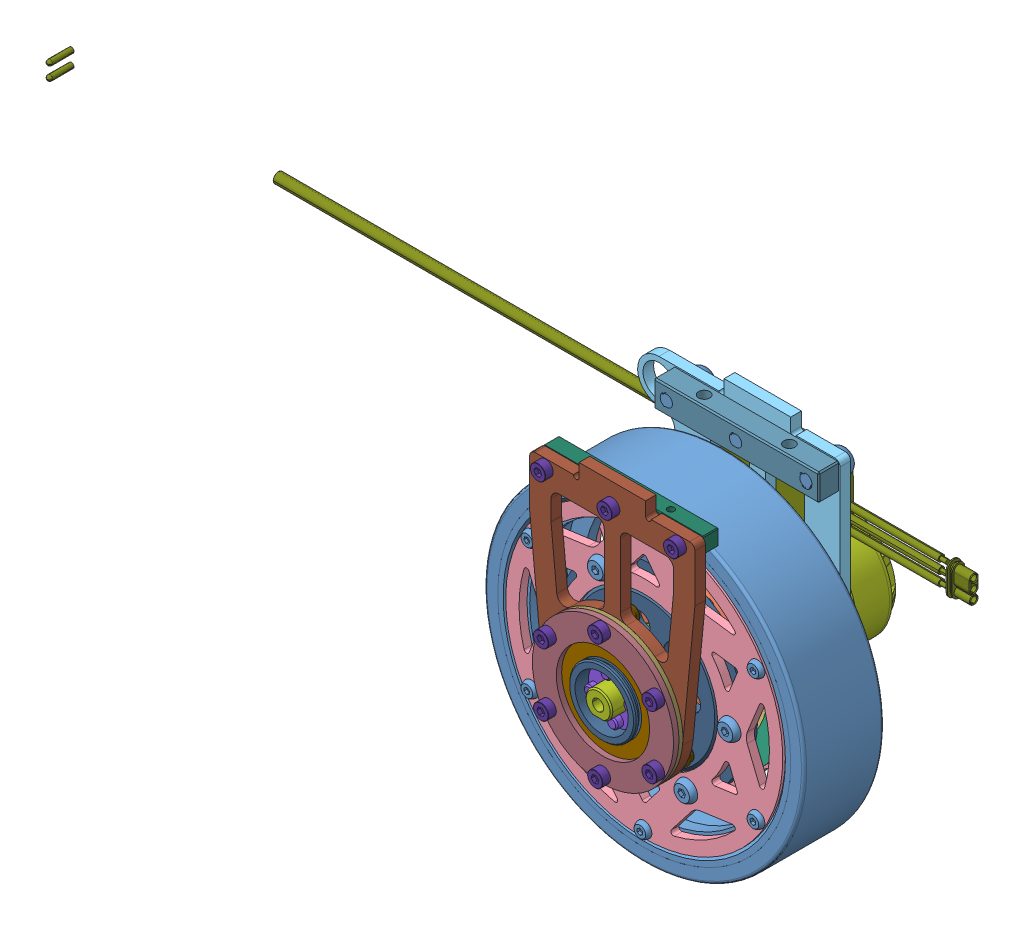
SolidWorks assembly 驱动轮部分, configuration 默认. Lengths in mm.
Overall size (142.07 142.07 99.6).
53 component instances, 19 part files, 115 mates.
Components (placement in the parent):
- 铝芯包胶轮-1: 铝芯包胶轮 [默认] at origin size (120 120 30)
- 3508电机座-1: 3508电机座 [默认] at (0 0 -27.5) x (1 0 0) z (0 -1 0) size (62 39.5 60.69)
- 薄型滚珠轴承6809zz45×58×7-1: 薄型滚珠轴承6809zz45×58×7 [默认] at (0 0 -12) x (0.929394 0.369089 0) z (0.369089 -0.929394 0) size (58 7 58)
- 舵轮盖板-内-1: 舵轮盖板-内 [内 ] at (0 0 -12) x (-0.5 -0.866025 0) z (0.866025 -0.5 0) size (104 3 104)
- 舵轮系基板-1: 舵轮系基板 [默认] at (0 0 -31.5) size (76 100.33 4)
- 舵轮系内侧轴承座-1: 舵轮系内侧轴承座 [默认] at (0 0 -5) x (0.5 0.866025 0) z (-0.866025 0.5 0) size (72 8 72)
- RoboMaster M3508直流无刷减速电机-1: RoboMaster M3508直流无刷减速电机 [默认] at (5.259 17.5861 -81.441) x (-0.925598 0.378508 0) z (0 0 1) size (42 42.01 98.4)
- 舵轮盖板-内-2: 舵轮盖板-内 [外] at (0 0 15) x (-0.5 -0.866025 0) z (0.866025 -0.5 0) size (104 3 104)
- 涨紧套Z21-10x20x13-1: 涨紧套Z21-10x20x13 [默认] at (0 0 13) x (0.985721 0.168386 0) z (0.168386 -0.985721 0) size (20 15.5 20)
- 法兰轴承-1: 法兰轴承 [25*37*7-1.5] at (0 0 28.5) x (0.417782 -0.908547 0) z (0.908547 0.417782 0) size (40 7 40)
- 轮组双端支撑件-1: 轮组双端支撑件 [默认] at (0 0 8) x (0.995882 0.09066 0) z (0.09066 -0.995882 0) size (70.95 23 70.95)
- 双端支撑板-1: 双端支撑板 [默认] at (0 0 23) size (62 96.5 4)
- 舵轮打印件垫片-1: 舵轮打印件垫片 [默认] at (0 0 27) size (53 53 1.5)
- 轮组压板-1: 轮组压板 [默认] at (0 0 28.5) size (53 53 2)
- 舵轮铝条直角连接件-2: 舵轮铝条直角连接件 [默认] at (0 60 -23.5) size (62 10 8)
- 双端支撑铝条-1: 双端支撑铝条 [默认] at (0 62 20) size (60 6 6)
- C620无刷电机调速器-1: C620无刷电机调速器 [默认] at (1.7 41 -36.9) x (1 0 0) z (0 -1 0) size (59.4 11.5 26.13)
- 12.9级圆柱头螺钉-4: 12.9级圆柱头螺钉 [M3*10] at (25 62 30) x (0.999644 -0.026698 0) z (0 0 1) size (5.68 5.68 13)
- 12.9级圆柱头螺钉-5: 12.9级圆柱头螺钉 [M3*10] at (0 62 30) x (0.999644 -0.026698 0) z (0 0 1) size (5.68 5.68 13)
- 12.9级圆柱头螺钉-6: 12.9级圆柱头螺钉 [M3*10] at (-25 62 30) x (0.999644 -0.026698 0) z (0 0 1) size (5.68 5.68 13)
- 12.9级圆柱头螺钉-7: 12.9级圆柱头螺钉 [M3*12] at (-20.3516 11.75 33.5) x (0.999644 -0.026698 0) z (0 0 1) size (5.68 5.68 15)
- 百瑞特防滑螺母-1: 百瑞特防滑螺母 [M3] at (-20.3516 11.75 20.6) x (0.875007 -0.48411 0) z (-0.48411 -0.875007 0) size (5.5 3.9 6.35)
- 12.9级圆柱头螺钉-8: 12.9级圆柱头螺钉 [M3*12] at (-20.3516 -11.75 33.5) x (0.991232 0.132136 0) z (0 0 1) size (5.68 5.68 15)
- 百瑞特防滑螺母-2: 百瑞特防滑螺母 [M3] at (-20.3516 -11.75 20.6) x (0.940696 -0.339252 0) z (-0.339252 -0.940696 0) size (5.5 3.9 6.35)
- 12.9级圆柱头螺钉-9: 12.9级圆柱头螺钉 [M3*12] at (0 -23.5 33.5) x (0.966338 0.257276 0) z (0 0 1) size (5.68 5.68 15)
- 百瑞特防滑螺母-3: 百瑞特防滑螺母 [M3] at (0 -23.5 20.6) x (0.976236 -0.216709 0) z (-0.216709 -0.976236 0) size (5.5 3.9 6.35)
- 12.9级圆柱头螺钉-10: 12.9级圆柱头螺钉 [M3*12] at (20.3516 -11.75 33.5) x (0.93815 0.34623 0) z (0 0 1) size (5.68 5.68 15)
- 百瑞特防滑螺母-4: 百瑞特防滑螺母 [M3] at (20.3516 -11.75 20.6) x (0.992186 -0.124769 0) z (-0.124769 -0.992186 0) size (5.5 3.9 6.35)
- 12.9级圆柱头螺钉-11: 12.9级圆柱头螺钉 [M3*12] at (20.3516 11.75 33.5) x (0.91791 0.396788 0) z (0 0 1) size (5.68 5.68 15)
- 百瑞特防滑螺母-5: 百瑞特防滑螺母 [M3] at (20.3516 11.75 20.6) x (0.997507 -0.07057 0) z (-0.07057 -0.997507 0) size (5.5 3.9 6.35)
- 12.9级圆柱头螺钉-12: 12.9级圆柱头螺钉 [M3*12] at (0 23.5 33.5) x (0.914007 0.405699 0) z (0 0 1) size (5.68 5.68 15)
- 百瑞特防滑螺母-6: 百瑞特防滑螺母 [M3] at (0 23.5 20.6) x (0.998146 -0.060863 0) z (-0.060863 -0.998146 0) size (5.5 3.9 6.35)
- 12.9级圆柱头螺钉-14: 12.9级圆柱头螺钉 [M4*10] at (19.4454 -19.4454 -35.5) x (-0.999764 -0.021708 0) z (0 0 -1) size (7.22 7.22 14)
- 12.9级圆柱头螺钉-15: 12.9级圆柱头螺钉 [M4*10] at (27.5 0 -35.5) x (-0.999764 -0.021708 0) z (0 0 -1) size (7.22 7.22 14)
- 12.9级圆柱头螺钉-16: 12.9级圆柱头螺钉 [M4*10] at (19.4454 19.4454 -35.5) x (-0.999764 -0.021708 0) z (0 0 -1) size (7.22 7.22 14)
- 12.9级圆柱头螺钉-17: 12.9级圆柱头螺钉 [M4*10] at (-19.4454 -19.4454 -35.5) x (-0.999764 -0.021708 0) z (0 0 -1) size (7.22 7.22 14)
- 12.9级圆柱头螺钉-18: 12.9级圆柱头螺钉 [M4*10] at (-27.5 0 -35.5) x (-0.999764 -0.021708 0) z (0 0 -1) size (7.22 7.22 14)
- 12.9级圆柱头螺钉-19: 12.9级圆柱头螺钉 [M4*10] at (-19.4454 19.4454 -35.5) x (-0.999764 -0.021708 0) z (0 0 -1) size (7.22 7.22 14)
- 10.9级半圆头螺栓-1: 10.9级半圆头螺栓 [M5*12] at (-26 60 -31.5) x (0.059849 -0.998207 0) z (-0.998207 -0.059849 0) size (9.5 14.75 9.5)
- 10.9级半圆头螺栓-2: 10.9级半圆头螺栓 [M5*12] at (26 60 -31.5) x (0.059849 -0.998207 0) z (-0.998207 -0.059849 0) size (9.5 14.75 9.5)
- 10.9级半圆头螺栓-3: 10.9级半圆头螺栓 [M5*12] at (0 60 -31.5) x (0.059849 -0.998207 0) z (-0.998207 -0.059849 0) size (9.5 14.75 9.5)
- 10.9级半圆头螺栓-4: 10.9级半圆头螺栓 [M4*8] at (-16.25 -28.1458 15) x (0.975246 0.221124 0) z (-0.221124 0.975246 0) size (7.6 10.2 7.6)
- 10.9级半圆头螺栓-5: 10.9级半圆头螺栓 [M4*8] at (16.25 -28.1458 15) x (0.975246 0.221124 0) z (-0.221124 0.975246 0) size (7.6 10.2 7.6)
- 10.9级半圆头螺栓-6: 10.9级半圆头螺栓 [M4*8] at (32.5 0 15) x (0.975246 0.221124 0) z (-0.221124 0.975246 0) size (7.6 10.2 7.6)
- 10.9级半圆头螺栓-7: 10.9级半圆头螺栓 [M4*8] at (16.25 28.1458 15) x (0.92785 0.372955 0) z (-0.372955 0.92785 0) size (7.6 10.2 7.6)
- 10.9级半圆头螺栓-8: 10.9级半圆头螺栓 [M4*8] at (-16.25 28.1458 15) x (0.872808 0.488064 0) z (-0.488064 0.872808 0) size (7.6 10.2 7.6)
- 10.9级半圆头螺栓-9: 10.9级半圆头螺栓 [M4*8] at (-32.5 0 15) x (0.823514 0.567296 0) z (-0.567296 0.823514 0) size (7.6 10.2 7.6)
- 10.9级半圆头螺栓-11: 10.9级半圆头螺栓 [M3*8] at (-42.4352 24.5 15) x (0.243917 0.969796 0) z (-0.969796 0.243917 0) size (5.7 9.65 5.7)
- 10.9级半圆头螺栓-13: 10.9级半圆头螺栓 [M3*8] at (-42.4352 -24.5 15) x (0.087067 0.996202 0) z (-0.996202 0.087067 0) size (5.7 9.65 5.7)
- 10.9级半圆头螺栓-14: 10.9级半圆头螺栓 [M3*8] at (0 -49 15) x (-0.04049 0.99918 0) z (-0.99918 -0.04049 0) size (5.7 9.65 5.7)
- 10.9级半圆头螺栓-15: 10.9级半圆头螺栓 [M3*8] at (42.4352 -24.5 15) x (-0.133449 0.991056 0) z (-0.991056 -0.133449 0) size (5.7 9.65 5.7)
- 10.9级半圆头螺栓-16: 10.9级半圆头螺栓 [M3*8] at (42.4352 24.5 15) x (-0.187203 0.982321 0) z (-0.982321 -0.187203 0) size (5.7 9.65 5.7)
- 10.9级半圆头螺栓-17: 10.9级半圆头螺栓 [M3*8] at (0 49 15) x (-0.19675 0.980454 0) z (-0.980454 -0.19675 0) size (5.7 9.65 5.7)
Mates (geometry in assembly coordinates):
- 同心1: concentric aligned: cylinder of 铝芯包胶轮-1 through (0 0 12) axis (0 0 1) radius 52; cylinder of 舵轮盖板-内-1 through (0 0 -15) axis (0 0 1) radius 27.5
- 重合1: coincident anti-aligned: plane of 铝芯包胶轮-1 through (0 0 -12) normal (0 0 -1); plane of 舵轮盖板-内-1 through (0 0 -12) normal (0 0 1)
- 同心2: concentric aligned: cylinder of 铝芯包胶轮-1 through (-42.4352 24.5 12) axis (0 0 1) radius 1.25; cylinder of 舵轮盖板-内-1 through (-42.4352 24.5 -15) axis (0 0 1) radius 1.525
- 同心3: concentric anti-aligned: cylinder of 3508电机座-1 through (0 0 -27.5) axis (0 0 -1) radius 22.5; cylinder of 舵轮盖板-内-1 through (0 0 -15) axis (0 0 1) radius 27.5
- 同心4: concentric aligned: cylinder of 3508电机座-1 through (0 0 -27.5) axis (0 0 -1) radius 22.5; cylinder of 薄型滚珠轴承6809zz45×58×7-1 through (0 0 -5) axis (0 0 -1) radius 22.5
- 重合2: coincident anti-aligned: plane of 3508电机座-1 through (-24 0 -12) normal (0 0 1); plane of 薄型滚珠轴承6809zz45×58×7-1 through (0 0 -12) normal (0 0 -1)
- 重合3: coincident anti-aligned: plane of 薄型滚珠轴承6809zz45×58×7-1 through (0 0 -12) normal (0 0 -1); plane of 舵轮盖板-内-1 through (0 0 -12) normal (0 0 1)
- 平行1: parallel aligned: plane of 舵轮系基板-1 through (31 65 -27.5) normal (1 0 0)
- 同心5: concentric aligned: cylinder of 3508电机座-1 through (0 0 -27.5) axis (0 0 -1) radius 24; cylinder of 舵轮系基板-1 through (0 0 -27.5) axis (0 0 -1) radius 24
- 重合4: coincident anti-aligned: plane of 3508电机座-1 through (-31 0 -27.5) normal (0 0 -1); plane of 舵轮系基板-1 through (0 0 -27.5) normal (0 0 1)
- 同心6: concentric anti-aligned: cylinder of 薄型滚珠轴承6809zz45×58×7-1 through (0 0 -5) axis (0 0 -1) radius 29; cylinder of 舵轮系内侧轴承座-1 through (0 0 -12) axis (0 0 1) radius 36
- 重合5: coincident anti-aligned: plane of 薄型滚珠轴承6809zz45×58×7-1 through (0 0 -5) normal (0 0 1); plane of 舵轮系内侧轴承座-1 through (0 0 -5) normal (0 0 -1)
- 同心7: concentric anti-aligned: cylinder of 舵轮盖板-内-1 through (16.25 28.1458 -15) axis (0 0 1) radius 2; cylinder of 舵轮系内侧轴承座-1 through (16.25 28.1458 -12) axis (0 0 -1) radius 1.65
- 同心9: concentric anti-aligned: cylinder of 3508电机座-1 through (19.4454 -19.4454 -22.5) axis (0 0 1) radius 1.65; cylinder of 舵轮系基板-1 through (19.4454 -19.4454 -27.5) axis (0 0 -1) radius 2
- 同心10: concentric aligned: cylinder of 3508电机座-1 through (0 0 -27.5) axis (0 0 -1) radius 21; cylinder of RoboMaster M3508直流无刷减速电机-1 through (0 0 -31) axis (0 0 -1) radius 21
- 重合6: coincident anti-aligned: plane of 3508电机座-1 through (-21 0 5) normal (0 0 -1); plane of RoboMaster M3508直流无刷减速电机-1 through (9.1924 9.1924 5) normal (0 0 1)
- 同心11: concentric aligned: cylinder of 3508电机座-1 through (0 17.5 8) axis (0 0 1) radius 2; cylinder of RoboMaster M3508直流无刷减速电机-1 through (0 17.5 5) axis (0 0 1) radius 1.65
- 同心12: concentric aligned: cylinder of RoboMaster M3508直流无刷减速电机-1 through (0 0 32.3) axis (0 0 1) radius 5; cylinder of 舵轮盖板-内-2 through (0 0 12) axis (0 0 1) radius 27.5
- 重合7: coincident anti-aligned: plane of 铝芯包胶轮-1 through (0 0 12) normal (0 0 1); plane of 舵轮盖板-内-2 through (0 0 12) normal (0 0 -1)
- 同心13: concentric aligned: cylinder of 铝芯包胶轮-1 through (0 49 12) axis (0 0 1) radius 1.25; cylinder of 舵轮盖板-内-2 through (0 49 12) axis (0 0 1) radius 1.525
- 同心14: concentric anti-aligned: cylinder of RoboMaster M3508直流无刷减速电机-1 through (0 0 32.3) axis (0 0 1) radius 5; cylinder of 涨紧套Z21-10x20x13-1 through (0 0 26) axis (0 0 -1) radius 5
- 同心15: concentric anti-aligned: cylinder of 涨紧套Z21-10x20x13-1 through (0 0 26) axis (0 0 -1) radius 10; cylinder of 法兰轴承-1 through (0 0 21.5) axis (0 0 1) radius 12.5
- 重合8: coincident anti-aligned: plane of 舵轮盖板-内-2 through (0 0 12) normal (0 0 -1); plane of 轮组双端支撑件-1 through (-27.3619 -2.4909 12) normal (0 0 1)
- 同心16: concentric anti-aligned: cylinder of RoboMaster M3508直流无刷减速电机-1 through (0 0 32.3) axis (0 0 1) radius 5; cylinder of 轮组双端支撑件-1 through (0 0 8) axis (0 0 -1) radius 12.5
- 距离1: distance = 5 mm aligned: plane of 涨紧套Z21-10x20x13-1 through (0 0 26) normal (0 0 1); plane of 轮组双端支撑件-1 through (-9.9588 -0.9066 31) normal (0 0 1)
- 重合9: coincident aligned: plane of 法兰轴承-1 through (0 0 28.5) normal (0 0 1); plane of 轮组双端支撑件-1 through (11.5522 1.0517 28.5) normal (0 0 1)
- 重合10: coincident anti-aligned: plane of 法兰轴承-1 through (0 0 27) normal (0 0 -1); plane of 双端支撑板-1 through (0 0 27) normal (0 0 1)
- 同心17: concentric anti-aligned: cylinder of 法兰轴承-1 through (0 0 21.5) axis (0 0 1) radius 18.5; cylinder of 双端支撑板-1 through (0 0 27) axis (0 0 -1) radius 18.5
- 平行2: parallel aligned: plane of 舵轮系基板-1 through (-31 0 -27.5) normal (-1 0 0); plane of 双端支撑板-1 through (-31 0 27) normal (-1 0 0)
- 同心18: concentric anti-aligned: cylinder of 法兰轴承-1 through (0 0 27) axis (0 0 1) radius 20; cylinder of 舵轮打印件垫片-1 through (0 0 28.5) axis (0 0 -1) radius 20.5
- 重合11: coincident anti-aligned: plane of 双端支撑板-1 through (0 0 27) normal (0 0 1); plane of 舵轮打印件垫片-1 through (0 0 27) normal (0 0 -1)
- 重合12: coincident aligned: plane of 舵轮打印件垫片-1 through (0 0 27) normal (0 1 0)
- 重合13: coincident anti-aligned: plane of 舵轮打印件垫片-1 through (0 0 28.5) normal (0 0 1); plane of 轮组压板-1 through (0 0 28.5) normal (0 0 -1)
- 同心19: concentric aligned: cylinder of 轮组双端支撑件-1 through (0 0 8) axis (0 0 -1) radius 10; cylinder of 轮组压板-1 through (0 0 30.5) axis (0 0 -1) radius 17.5
- 同心20: concentric aligned: cylinder of 舵轮打印件垫片-1 through (0 23.5 27) axis (0 0 1) radius 1.65; cylinder of 轮组压板-1 through (0 23.5 28.5) axis (0 0 1) radius 1.525
- 重合15: coincident anti-aligned: plane of 舵轮系基板-1 through (0 0 -27.5) normal (0 0 1); plane of 舵轮铝条直角连接件-2 through (0 60 -27.5) normal (0 0 -1)
- 同心22: concentric anti-aligned: cylinder of 舵轮系基板-1 through (26 60 -27.5) axis (0 0 -1) radius 2.5; cylinder of 舵轮铝条直角连接件-2 through (26 60 -19.5) axis (0 0 1) radius 2.1
- 重合16: coincident anti-aligned: plane of 双端支撑板-1 through (0 0 23) normal (0 0 -1); plane of 双端支撑铝条-1 through (0 62 23) normal (0 0 1)
- 重合17: coincident aligned: plane of 双端支撑板-1 through (-31 65 27) normal (0 1 0); plane of 双端支撑铝条-1 through (-30 65 23) normal (0 1 0)
- 宽度1: width aligned: plane of 双端支撑板-1 through (-31 0 27) normal (-1 0 0); plane of 双端支撑板-1 through (31 65 27) normal (1 0 0); plane of 双端支撑铝条-1 through (-30 59 23) normal (-1 0 0); plane of 双端支撑铝条-1 through (30 59 23) normal (1 0 0)
- 重合14: coincident anti-aligned: plane of 舵轮系基板-1 through (0 0 -31.5) normal (0 0 -1); plane of C620无刷电机调速器-1 through (0 41 -31.5) normal (0 0 1)
- 同心23: concentric aligned: cylinder of 舵轮系基板-1 through (22.6 50 -27.5) axis (0 0 -1) radius 1.1; cylinder of C620无刷电机调速器-1 through (22.6 50 -22) axis (0 0 -1) radius 1
- 同心24: concentric aligned: cylinder of 舵轮系基板-1 through (22.6 32 -27.5) axis (0 0 -1) radius 1.1; cylinder of C620无刷电机调速器-1 through (22.6 32 -22) axis (0 0 -1) radius 1
- 同心28: concentric anti-aligned: cylinder of 双端支撑板-1 through (25 62 5) axis (0 0 1) radius 1.525; cylinder of 12.9级圆柱头螺钉-4 through (25 62 17) axis (0 0 -1) radius 1.5
- 重合21: coincident anti-aligned: plane of 双端支撑板-1 through (0 0 27) normal (0 0 1); plane of 12.9级圆柱头螺钉-4 through (25.0758 64.839 27) normal (0 0 -1)
- 同心291: concentric anti-aligned: cylinder of 双端支撑板-1 through (0 62 5) axis (0 0 1) radius 1.525; cylinder of 12.9级圆柱头螺钉-5 through (0 62 17) axis (0 0 -1) radius 2.84
- 重合221: coincident anti-aligned: plane of 双端支撑板-1 through (0 0 27) normal (0 0 1); plane of 12.9级圆柱头螺钉-5 through (0.0758 64.839 27) normal (0 0 -1)
- 同心301: concentric anti-aligned: cylinder of 双端支撑板-1 through (-25 62 5) axis (0 0 1) radius 1.525; cylinder of 12.9级圆柱头螺钉-6 through (-25 62 17) axis (0 0 -1) radius 2.84
- 重合231: coincident anti-aligned: plane of 双端支撑板-1 through (0 0 27) normal (0 0 1); plane of 12.9级圆柱头螺钉-6 through (-24.9242 64.839 27) normal (0 0 -1)
- 同心31: concentric anti-aligned: cylinder of 轮组压板-1 through (-20.3516 11.75 28.5) axis (0 0 1) radius 1.525; cylinder of 12.9级圆柱头螺钉-7 through (-20.3516 11.75 18.5) axis (0 0 -1) radius 1.5
- 重合24: coincident anti-aligned: plane of 轮组压板-1 through (0 0 30.5) normal (0 0 1); plane of 12.9级圆柱头螺钉-7 through (-20.2758 14.589 30.5) normal (0 0 -1)
- 同心32: concentric aligned: cylinder of 12.9级圆柱头螺钉-7 through (-20.3516 11.75 18.5) axis (0 0 -1) radius 1.5; cylinder of 百瑞特防滑螺母-1 through (-20.3516 11.75 23) axis (0 0 -1) radius 1.5
- 重合25: coincident anti-aligned: plane of 双端支撑板-1 through (0 0 23) normal (0 0 -1); plane of 百瑞特防滑螺母-1 through (-20.3516 11.75 23) normal (0 0 1)
- 同心33: concentric aligned: cylinder of 12.9级圆柱头螺钉-8 through (-20.3516 -11.75 18.5) axis (0 0 -1) radius 1.5; cylinder of 百瑞特防滑螺母-2 through (-20.3516 -11.75 23) axis (0 0 -1) radius 1.5
- 重合26: coincident anti-aligned: plane of 轮组压板-1 through (0 0 30.5) normal (0 0 1); plane of 12.9级圆柱头螺钉-8 through (-20.7269 -8.9349 30.5) normal (0 0 -1)
- 重合27: coincident anti-aligned: plane of 双端支撑板-1 through (0 0 23) normal (0 0 -1); plane of 百瑞特防滑螺母-2 through (-20.3516 -11.75 23) normal (0 0 1)
- 同心34: concentric anti-aligned: cylinder of 轮组压板-1 through (-20.3516 -11.75 28.5) axis (0 0 1) radius 1.525; cylinder of 12.9级圆柱头螺钉-8 through (-20.3516 -11.75 18.5) axis (0 0 -1) radius 1.5
- 同心35: concentric aligned: cylinder of 12.9级圆柱头螺钉-9 through (0 -23.5 18.5) axis (0 0 -1) radius 1.5; cylinder of 百瑞特防滑螺母-3 through (0 -23.5 23) axis (0 0 -1) radius 1.5
- 重合28: coincident anti-aligned: plane of 轮组压板-1 through (0 0 30.5) normal (0 0 1); plane of 12.9级圆柱头螺钉-9 through (-0.7307 -20.7556 30.5) normal (0 0 -1)
- 重合29: coincident anti-aligned: plane of 双端支撑板-1 through (0 0 23) normal (0 0 -1); plane of 百瑞特防滑螺母-3 through (0 -23.5 23) normal (0 0 1)
- 同心36: concentric anti-aligned: cylinder of 轮组压板-1 through (0 -23.5 28.5) axis (0 0 1) radius 1.525; cylinder of 12.9级圆柱头螺钉-9 through (0 -23.5 18.5) axis (0 0 -1) radius 1.5
- 同心37: concentric aligned: cylinder of 12.9级圆柱头螺钉-10 through (20.3516 -11.75 18.5) axis (0 0 -1) radius 1.5; cylinder of 百瑞特防滑螺母-4 through (20.3516 -11.75 23) axis (0 0 -1) radius 1.5
- 重合30: coincident anti-aligned: plane of 轮组压板-1 through (0 0 30.5) normal (0 0 1); plane of 12.9级圆柱头螺钉-10 through (19.3683 -9.0857 30.5) normal (0 0 -1)
- 重合31: coincident anti-aligned: plane of 双端支撑板-1 through (0 0 23) normal (0 0 -1); plane of 百瑞特防滑螺母-4 through (20.3516 -11.75 23) normal (0 0 1)
- 同心38: concentric anti-aligned: cylinder of 轮组压板-1 through (20.3516 -11.75 28.5) axis (0 0 1) radius 1.525; cylinder of 12.9级圆柱头螺钉-10 through (20.3516 -11.75 18.5) axis (0 0 -1) radius 1.5
- 同心39: concentric aligned: cylinder of 12.9级圆柱头螺钉-11 through (20.3516 11.75 18.5) axis (0 0 -1) radius 1.5; cylinder of 百瑞特防滑螺母-5 through (20.3516 11.75 23) axis (0 0 -1) radius 1.5
- 重合32: coincident anti-aligned: plane of 轮组压板-1 through (0 0 30.5) normal (0 0 1); plane of 12.9级圆柱头螺钉-11 through (19.2247 14.3569 30.5) normal (0 0 -1)
- 重合33: coincident anti-aligned: plane of 双端支撑板-1 through (0 0 23) normal (0 0 -1); plane of 百瑞特防滑螺母-5 through (20.3516 11.75 23) normal (0 0 1)
- 同心40: concentric anti-aligned: cylinder of 轮组压板-1 through (20.3516 11.75 28.5) axis (0 0 1) radius 1.525; cylinder of 12.9级圆柱头螺钉-11 through (20.3516 11.75 18.5) axis (0 0 -1) radius 1.5
- 同心41: concentric aligned: cylinder of 12.9级圆柱头螺钉-12 through (0 23.5 18.5) axis (0 0 -1) radius 1.5; cylinder of 百瑞特防滑螺母-6 through (0 23.5 23) axis (0 0 -1) radius 1.5
- 重合34: coincident anti-aligned: plane of 轮组压板-1 through (0 0 30.5) normal (0 0 1); plane of 12.9级圆柱头螺钉-12 through (-1.1522 26.0958 30.5) normal (0 0 -1)
- 重合35: coincident anti-aligned: plane of 双端支撑板-1 through (0 0 23) normal (0 0 -1); plane of 百瑞特防滑螺母-6 through (0 23.5 23) normal (0 0 1)
- 同心42: concentric anti-aligned: cylinder of 轮组压板-1 through (0 23.5 28.5) axis (0 0 1) radius 1.525; cylinder of 12.9级圆柱头螺钉-12 through (0 23.5 18.5) axis (0 0 -1) radius 1.5
- 同心44: concentric anti-aligned: cylinder of 舵轮系基板-1 through (19.4454 -19.4454 -27.5) axis (0 0 -1) radius 2; cylinder of 12.9级圆柱头螺钉-14 through (19.4454 -19.4454 -21.5) axis (0 0 1) radius 2
- 重合38: coincident anti-aligned: plane of 舵轮系基板-1 through (0 0 -31.5) normal (0 0 -1); plane of 12.9级圆柱头螺钉-14 through (19.3671 -15.8363 -31.5) normal (0 0 1)
- 同心451: concentric anti-aligned: cylinder of 舵轮系基板-1 through (27.5 0 -27.5) axis (0 0 -1) radius 2; cylinder of 12.9级圆柱头螺钉-15 through (27.5 0 -21.5) axis (0 0 1) radius 3.61
- 重合391: coincident anti-aligned: plane of 舵轮系基板-1 through (0 0 -31.5) normal (0 0 -1); plane of 12.9级圆柱头螺钉-15 through (27.4216 3.6091 -31.5) normal (0 0 1)
- 同心461: concentric anti-aligned: cylinder of 舵轮系基板-1 through (19.4454 19.4454 -27.5) axis (0 0 -1) radius 2; cylinder of 12.9级圆柱头螺钉-16 through (19.4454 19.4454 -21.5) axis (0 0 1) radius 3.61
- 重合401: coincident anti-aligned: plane of 舵轮系基板-1 through (0 0 -31.5) normal (0 0 -1); plane of 12.9级圆柱头螺钉-16 through (19.3671 23.0546 -31.5) normal (0 0 1)
- 同心471: concentric anti-aligned: cylinder of 舵轮系基板-1 through (-19.4454 -19.4454 -27.5) axis (0 0 -1) radius 2; cylinder of 12.9级圆柱头螺钉-17 through (-19.4454 -19.4454 -21.5) axis (0 0 1) radius 3.61
- 重合411: coincident anti-aligned: plane of 舵轮系基板-1 through (0 0 -31.5) normal (0 0 -1); plane of 12.9级圆柱头螺钉-17 through (-19.5238 -15.8363 -31.5) normal (0 0 1)
- 同心481: concentric anti-aligned: cylinder of 舵轮系基板-1 through (-27.5 0 -27.5) axis (0 0 -1) radius 2; cylinder of 12.9级圆柱头螺钉-18 through (-27.5 0 -21.5) axis (0 0 1) radius 3.61
- 重合421: coincident anti-aligned: plane of 舵轮系基板-1 through (0 0 -31.5) normal (0 0 -1); plane of 12.9级圆柱头螺钉-18 through (-27.5784 3.6091 -31.5) normal (0 0 1)
- 同心491: concentric anti-aligned: cylinder of 舵轮系基板-1 through (-19.4454 19.4454 -27.5) axis (0 0 -1) radius 2; cylinder of 12.9级圆柱头螺钉-19 through (-19.4454 19.4454 -21.5) axis (0 0 1) radius 3.61
- 重合431: coincident anti-aligned: plane of 舵轮系基板-1 through (0 0 -31.5) normal (0 0 -1); plane of 12.9级圆柱头螺钉-19 through (-19.5238 23.0546 -31.5) normal (0 0 1)
- 同心50: concentric aligned: cylinder of 舵轮系基板-1 through (-26 60 -27.5) axis (0 0 -1) radius 2.5; cylinder of 10.9级半圆头螺栓-1 through (-26 60 -19.5) axis (0 0 -1) radius 2.5
- 重合44: coincident anti-aligned: plane of 舵轮系基板-1 through (0 0 -31.5) normal (0 0 -1); plane of 10.9级半圆头螺栓-1 through (-26 60 -31.5) normal (0 0 1)
- 同心51: concentric aligned: cylinder of 舵轮系基板-1 through (26 60 -27.5) axis (0 0 -1) radius 2.5; cylinder of 10.9级半圆头螺栓-2 through (26 60 -19.5) axis (0 0 -1) radius 2.5
- 重合45: coincident anti-aligned: plane of 舵轮系基板-1 through (0 0 -31.5) normal (0 0 -1); plane of 10.9级半圆头螺栓-2 through (26 60 -31.5) normal (0 0 1)
- 同心52: concentric aligned: cylinder of 舵轮系基板-1 through (0 60 -27.5) axis (0 0 -1) radius 2.5; cylinder of 10.9级半圆头螺栓-3 through (0 60 -19.5) axis (0 0 -1) radius 2.5
- 重合46: coincident anti-aligned: plane of 舵轮系基板-1 through (0 0 -31.5) normal (0 0 -1); plane of 10.9级半圆头螺栓-3 through (0 60 -31.5) normal (0 0 1)
- 同心492: concentric aligned: cylinder of 舵轮盖板-内-2 through (-16.25 -28.1458 12) axis (0 0 1) radius 2; cylinder of 10.9级半圆头螺栓-4 through (-16.25 -28.1458 7) axis (0 0 1) radius 2
- 重合432: coincident anti-aligned: plane of 舵轮盖板-内-2 through (0 0 15) normal (0 0 1); plane of 10.9级半圆头螺栓-4 through (-16.25 -28.1458 15) normal (0 0 -1)
- 同心493: concentric aligned: cylinder of 舵轮盖板-内-2 through (16.25 -28.1458 12) axis (0 0 1) radius 2; cylinder of 10.9级半圆头螺栓-5 through (16.25 -28.1458 7) axis (0 0 1) radius 2
- 重合433: coincident anti-aligned: plane of 舵轮盖板-内-2 through (0 0 15) normal (0 0 1); plane of 10.9级半圆头螺栓-5 through (16.25 -28.1458 15) normal (0 0 -1)
- 同心494: concentric aligned: cylinder of 舵轮盖板-内-2 through (32.5 0 12) axis (0 0 1) radius 2; cylinder of 10.9级半圆头螺栓-6 through (32.5 0 7) axis (0 0 1) radius 2
- 重合434: coincident anti-aligned: plane of 舵轮盖板-内-2 through (0 0 15) normal (0 0 1); plane of 10.9级半圆头螺栓-6 through (32.5 0 15) normal (0 0 -1)
- 重合435: coincident anti-aligned: plane of 舵轮盖板-内-2 through (0 0 15) normal (0 0 1); plane of 10.9级半圆头螺栓-7 through (16.25 28.1458 15) normal (0 0 -1)
- 同心495: concentric aligned: cylinder of 舵轮盖板-内-2 through (16.25 28.1458 12) axis (0 0 1) radius 2; cylinder of 10.9级半圆头螺栓-7 through (16.25 28.1458 7) axis (0 0 1) radius 2
- 重合436: coincident anti-aligned: plane of 舵轮盖板-内-2 through (0 0 15) normal (0 0 1); plane of 10.9级半圆头螺栓-8 through (-16.25 28.1458 15) normal (0 0 -1)
- 同心496: concentric aligned: cylinder of 舵轮盖板-内-2 through (-16.25 28.1458 12) axis (0 0 1) radius 2; cylinder of 10.9级半圆头螺栓-8 through (-16.25 28.1458 7) axis (0 0 1) radius 2
- 重合437: coincident anti-aligned: plane of 舵轮盖板-内-2 through (0 0 15) normal (0 0 1); plane of 10.9级半圆头螺栓-9 through (-32.5 0 15) normal (0 0 -1)
- 同心497: concentric aligned: cylinder of 舵轮盖板-内-2 through (-32.5 0 12) axis (0 0 1) radius 2; cylinder of 10.9级半圆头螺栓-9 through (-32.5 0 7) axis (0 0 1) radius 2
- 同心498: concentric aligned: cylinder of 舵轮盖板-内-2 through (-42.4352 24.5 12) axis (0 0 1) radius 1.525; cylinder of 10.9级半圆头螺栓-11 through (-42.4352 24.5 7) axis (0 0 1) radius 1.5
- 重合439: coincident anti-aligned: plane of 舵轮盖板-内-2 through (0 0 15) normal (0 0 1); plane of 10.9级半圆头螺栓-11 through (-42.4352 24.5 15) normal (0 0 -1)
- 重合440: coincident anti-aligned: plane of 舵轮盖板-内-2 through (0 0 15) normal (0 0 1); plane of 10.9级半圆头螺栓-13 through (-42.4352 -24.5 15) normal (0 0 -1)
- 同心499: concentric aligned: cylinder of 舵轮盖板-内-2 through (-42.4352 -24.5 12) axis (0 0 1) radius 1.525; cylinder of 10.9级半圆头螺栓-13 through (-42.4352 -24.5 7) axis (0 0 1) radius 1.5
- 重合441: coincident anti-aligned: plane of 舵轮盖板-内-2 through (0 0 15) normal (0 0 1); plane of 10.9级半圆头螺栓-14 through (0 -49 15) normal (0 0 -1)
- 同心500: concentric aligned: cylinder of 舵轮盖板-内-2 through (0 -49 12) axis (0 0 1) radius 1.525; cylinder of 10.9级半圆头螺栓-14 through (0 -49 7) axis (0 0 1) radius 1.5
- 重合442: coincident anti-aligned: plane of 舵轮盖板-内-2 through (0 0 15) normal (0 0 1); plane of 10.9级半圆头螺栓-15 through (42.4352 -24.5 15) normal (0 0 -1)
- 同心501: concentric aligned: cylinder of 舵轮盖板-内-2 through (42.4352 -24.5 12) axis (0 0 1) radius 1.525; cylinder of 10.9级半圆头螺栓-15 through (42.4352 -24.5 7) axis (0 0 1) radius 1.5
- 重合443: coincident anti-aligned: plane of 舵轮盖板-内-2 through (0 0 15) normal (0 0 1); plane of 10.9级半圆头螺栓-16 through (42.4352 24.5 15) normal (0 0 -1)
- 同心502: concentric aligned: cylinder of 舵轮盖板-内-2 through (42.4352 24.5 12) axis (0 0 1) radius 1.525; cylinder of 10.9级半圆头螺栓-16 through (42.4352 24.5 7) axis (0 0 1) radius 1.5
- 重合444: coincident anti-aligned: plane of 舵轮盖板-内-2 through (0 0 15) normal (0 0 1); plane of 10.9级半圆头螺栓-17 through (0 49 15) normal (0 0 -1)
- 同心503: concentric aligned: cylinder of 舵轮盖板-内-2 through (0 49 12) axis (0 0 1) radius 1.525; cylinder of 10.9级半圆头螺栓-17 through (0 49 7) axis (0 0 1) radius 1.5
